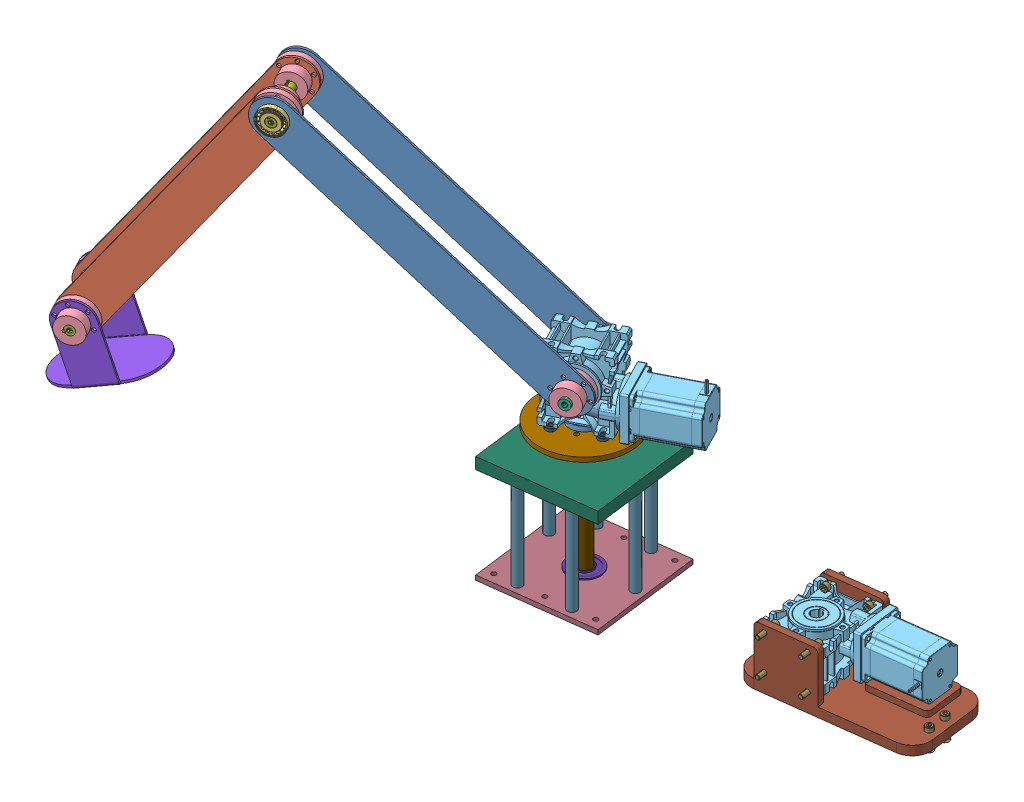
SolidWorks assembly Arm Assembly, configuration Default. Lengths in mm.
Overall size (1001.94 583.28 438.03).
58 component instances, 21 part files, 110 mates.
Components (placement in the parent):
- Link 2-1: Link 2 [Default] at (-10.4598 341.8399 327.9518) x (-0.673407 0.654009 0.344667) z (0.455616 0 0.890177) size (457.2 50.8 3.17)
- Link 3-1: Link 3 [Default] at (-284.4232 603.1069 549.3919) x (-0.514915 -0.815724 0.263547) z (0.455616 0 0.890177) size (406.4 50.8 3.17)
- Flanged Bearing-1: Flanged Bearing [Default] at (-472.9101 298.3431 587.1163) x (0.890177 0 -0.455616) z (0.455616 0 0.890177) size (38.1 38.1 12.7)
- Keyed hub-1: Keyed hub [Default] at (11.7089 322.6251 407.7249) x (0.874279 -0.188145 -0.447479) z (-0.167482 -0.982141 0.085722) size (50.8 25.4 50.8)
- Link 2-2: Link 2 [Default] at (30.1128 341.8399 407.2221) x (-0.673407 0.654009 0.344667) z (0.455616 0 0.890177) size (457.2 50.8 3.17)
- Link 3-2: Link 3 [Default] at (-309.7315 603.1069 499.9449) x (-0.514915 -0.815724 0.263547) z (0.455616 0 0.890177) size (406.4 50.8 3.17)
- Flanged Bearing-2: Flanged Bearing [Default] at (-256.8658 588.4145 557.7576) x (-0.847522 0.30584 0.433784) z (0.455616 0 0.890177) size (38.1 38.1 12.7)
- Flanged Bearing-3: Flanged Bearing [Default] at (-449.1178 298.3431 633.6014) x (-0.822281 -0.383049 0.420865) z (-0.455616 0 -0.890177) size (38.1 38.1 12.7)
- Keyed hub-2: Keyed hub [Default] at (-294.904 588.4145 483.4391) x (0.808999 0.417217 -0.414067) z (0.371397 -0.908807 -0.190091) size (50.8 25.4 50.8)
- Keyed hub-3: Keyed hub [Default] at (-20.1842 322.6251 345.4125) x (-0.874279 0.188145 0.447479) z (-0.167482 -0.982141 0.085722) size (50.8 25.4 50.8)
- Keyed hub-4: Keyed hub [Default] at (-260.9162 588.4145 549.8439) x (-0.808999 -0.417217 0.414067) z (0.371397 -0.908807 -0.190091) size (50.8 25.4 50.8)
- Flanged Bearing-4: Flanged Bearing [Default] at (-298.9544 588.4145 475.5254) x (0.819706 0.38995 -0.419547) z (-0.455616 0 -0.890177) size (38.1 38.1 12.7)
- Nema Stepper Motor-2: Nema Stepper Motor [Default] at (62.3488 303.6559 342.488) x (0.890177 0 -0.455616) z (-0.455616 0 -0.890177) size (171.01 100.01 63.01)
- Keyed Drive Shaft-1: Keyed Drive Shaft [Default] at (-60.5067 325.1756 260.6501) x (0.874279 -0.188145 -0.447479) z (0.455616 0 0.890177) size (19.9 19.9 128.01)
- Keyed Shaft-1: Keyed Shaft [Default] at (-306.0495 588.4145 461.663) x (0.808999 0.417217 -0.414067) z (0.455616 0 0.890177) size (12.7 12.5 104.14)
- Link 4-1: Link 4 [Default] at (-461.4839 217.0007 611.6395) x (0.455616 0 0.890177) z (-0.848146 -0.303649 0.434103) size (90.37 102.6 133.86)
- Keyed hub-5: Keyed hub [Default] at (-476.1168 298.3431 580.8511) x (0.270301 -0.952784 -0.138347) z (0.848146 0.303649 -0.434103) size (50.8 25.4 50.8)
- Keyed hub-6: Keyed hub [Default] at (-445.0674 298.3431 641.515) x (-0.270301 0.952784 0.138347) z (0.848146 0.303649 -0.434103) size (50.8 25.4 50.8)
- Keyed Shaft-2: Keyed Shaft [Default] at (-428.8657 298.3431 673.1697) x (0.270301 -0.952784 -0.138347) z (-0.455616 0 -0.890177) size (12.7 12.5 104.14)
- Joint 2 Motor Plate-1: Joint 2 Motor Plate [Default] at (-4.244 255.2751 376.7854) x (0.954214 0 0.299124) z (-0.299124 0 0.954214) size (127 6.35 127)
- 4 mm M6 spacer-1: 4 mm M6 spacer [94669A162] at (30.7255 263.6251 385.848) x (-0.888418 0 -0.459036) z (0 -1 0) size (13 13 4)
- 4 mm M6 spacer-2: 4 mm M6 spacer [94669A162] at (-17.344 263.6251 410.4513) x (0.999963 0 0.008554) z (0 -1 0) size (13 13 4)
- 4 mm M6 spacer-3: 4 mm M6 spacer [94669A162] at (8.8559 263.6251 343.1196) x (1 0 0) z (0 -1 0) size (13 13 4)
- 4 mm M6 spacer-4: 4 mm M6 spacer [94669A162] at (-39.2136 263.6251 367.7228) x (1 0 0) z (0 -1 0) size (13 13 4)
- Motor Mount Joint 1 Assembly-1: Motor Mount Joint 1 Assembly [Default] at (255.7253 -1.2672 148.6448) x (0.992107 0 -0.125391) z (0.125391 0 0.992107) size (228.6 94.85 140.08)
  - Joint 1 Motor Holder Bracket-1: Joint 1 Motor Holder Bracket [Default] at (55.8829 79.1234 191.166) size (228.6 82.55 114.78)
  - Nema Stepper Motor-1: Nema Stepper Motor [Default] at (81.7887 128.4828 180.6968) x (1 0 0) z (0 1 0) size (171.01 100.01 63.01)
  - Flanged Bearing-1: Flanged Bearing [Default] at (6.9829 88.5722 199.666) x (0.99323 0 0.116162) z (0 -1 0) size (38.1 38.1 12.7)
  - socket head cap screw_am-7: socket head cap screw_am [B18.3.1M - 6 x 1.0 x 25 Hex SHCS -- 25NHX] at (-20.0631 152.4828 153.666) x (0 0 -1) z (0.990069 0.140585 0) size (31 10 10)
  - socket head cap screw_am-8: socket head cap screw_am [B18.3.1M - 6 x 1.0 x 25 Hex SHCS -- 25NHX] at (33.9369 152.4828 228.666) x (0 0 1) z (-1 0 0) size (31 10 10)
  - socket head cap screw_am-9: socket head cap screw_am [B18.3.1M - 6 x 1.0 x 25 Hex SHCS -- 25NHX] at (-20.0631 152.4828 228.666) x (0 0 1) z (0.381849 0.924225 0) size (31 10 10)
  - socket head cap screw_am-10: socket head cap screw_am [B18.3.1M - 6 x 1.0 x 25 Hex SHCS -- 25NHX] at (-20.0631 104.4828 153.666) x (0 0 -1) z (0.756248 0.654286 0) size (31 10 10)
  - socket head cap screw_am-11: socket head cap screw_am [B18.3.1M - 6 x 1.0 x 25 Hex SHCS -- 25NHX] at (33.9369 104.4828 150.5881) x (0 0 -1) z (0.923728 0.383049 0) size (31 10 10)
  - socket head cap screw_am-12: socket head cap screw_am [B18.3.1M - 6 x 1.0 x 25 Hex SHCS -- 25NHX] at (-45.7171 97.8234 212.366) x (0 -1 0) z (-0.546944 0 0.837169) size (31 10 10)
  - socket head cap screw_am-19: socket head cap screw_am [B18.3.1M - 6 x 1.0 x 25 Hex SHCS -- 25NHX] at (-45.7171 97.8234 186.966) x (0 -1 0) z (-0.546944 0 0.837169) size (31 10 10)
  - socket head cap screw_am-14: socket head cap screw_am [B18.3.1M - 6 x 1.0 x 25 Hex SHCS -- 25NHX] at (33.9369 152.4828 153.666) x (0 0 -1) z (0.923728 0.383049 0) size (31 10 10)
  - socket head cap screw_am-15: socket head cap screw_am [B18.3.1M - 6 x 1.0 x 25 Hex SHCS -- 25NHX] at (157.4829 97.8234 186.966) x (0 -1 0) z (-0.546944 0 0.837169) size (31 10 10)
  - socket head cap screw_am-16: socket head cap screw_am [B18.3.1M - 6 x 1.0 x 25 Hex SHCS -- 25NHX] at (-20.0631 104.4828 228.666) x (0 0 1) z (-1 0 0) size (31 10 10)
  - socket head cap screw_am-17: socket head cap screw_am [B18.3.1M - 6 x 1.0 x 25 Hex SHCS -- 25NHX] at (33.9369 104.4828 228.666) x (0 0 1) z (-1 0 0) size (31 10 10)
  - socket head cap screw_am-18: socket head cap screw_am [B18.3.1M - 6 x 1.0 x 25 Hex SHCS -- 25NHX] at (157.4829 97.8234 212.366) x (0 -1 0) z (-0.546944 0 0.837169) size (31 10 10)
- Joint 1 bottom plate-1: Joint 1 bottom plate [89155K113] at (-4.244 81.0311 376.7854) x (-0.125391 0 -0.992107) z (0.992107 0 -0.125391) size (152.4 6.35 152.4)
- Base post-1: Base post [8974K269] at (21.393 160.4061 309.54) x (-0.837169 0 -0.546944) z (0 -1 0) size (12.7 12.7 127)
- Base post-2: Base post [8974K269] at (-29.8811 160.4061 444.0308) x (-0.837169 0 -0.546944) z (0 -1 0) size (12.7 12.7 127)
- Base post-3: Base post [8974K269] at (37.3177 160.4061 435.5376) x (0.463623 0 0.886032) z (0 -1 0) size (12.7 12.7 127)
- Base post-4: Base post [8974K269] at (58.7548 160.4061 368.8231) x (-0.837169 0 -0.546944) z (0 -1 0) size (12.7 12.7 127)
- Base post-5: Base post [8974K269] at (-70.4278 160.4061 359.5483) x (-0.837169 0 -0.546944) z (0 -1 0) size (12.7 12.7 127)
- Base post-6: Base post [8974K269] at (-45.8058 160.4061 318.0332) x (-0.837169 0 -0.546944) z (0 -1 0) size (12.7 12.7 127)
- Base post-7: Base post [8974K269] at (-64.0579 160.4061 409.9473) x (-0.837169 0 -0.546944) z (0 -1 0) size (12.7 12.7 127)
- Joint 1 top plate-1: Joint 1 top plate [89155K143] at (-4.244 219.1436 376.7854) x (-0.125391 0 -0.992107) z (0.992107 0 -0.125391) size (152.4 15.88 152.4)
- Tapered-Roller Bearing-1: Tapered-Roller Bearing [5709K77] at (-4.244 223.5886 376.7854) x (1 0 0) z (0 -1 0) size (45.24 45.24 17.1)
- base Ball Bearing 0.75 in-1: base Ball Bearing 0.75 in [6384K367] at (-4.244 79.4436 376.7854) x (1 0 0) z (0 -1 0) size (44.45 44.45 14.27)
- keyed shaft 0.75 in bore 9 in-1: keyed shaft 0.75 in bore 9 in [Default] at (-4.244 155.2626 376.7854) x (0.954214 0 0.299124) z (0 -1 0) size (19.05 18.75 228.6)
- 0.75 in shaft hub-1: 0.75 in shaft hub [Default] at (-4.244 248.9251 376.7854) x (-0.954214 0 -0.299124) z (0 -1 0) size (63.5 63.5 19.49)
- Clamping Two-Piece Shaft Collar 0.75 in-1: Clamping Two-Piece Shaft Collar 0.75 in [6436K16] at (-4.244 240.9876 376.7854) x (0.996685 0 0.081358) z (0 1 0) size (38.06 38.1 12.77)
- T-slot Slider-1: T-slot Slider [5278N52] at (236.9979 67.7205 365.0672) x (-0.837169 0 -0.546944) z (0 1 0) size (10 9.8 4.82)
- T-slot Slider-2: T-slot Slider [5278N52] at (233.8129 65.4156 339.8677) x (-0.837169 0 -0.546944) z (0 1 0) size (10 9.8 4.82)
- T-slot Slider-3: T-slot Slider [5278N52] at (438.5941 68.7454 339.5877) x (-0.838988 0 -0.544149) z (0 1 0) size (10 9.8 4.82)
- T-slot Slider-4: T-slot Slider [5278N52] at (435.4091 66.889 314.3882) x (-0.837169 0 -0.546944) z (0 1 0) size (10 9.8 4.82)
Mates (geometry in assembly coordinates):
- Concentric3: concentric aligned: cylinder of Keyed hub-1 through (15.3253 322.6251 414.7907) axis (0.455616 0 0.890177) radius 17.4625; cylinder of Link 2-2 through (15.3253 322.6251 414.7907) axis (0.455616 0 0.890177) radius 17.4625
- Coincident2: coincident anti-aligned: plane of Keyed hub-1 through (15.3253 322.6251 414.7907) normal (0.455616 0 0.890177); plane of Link 2-2 through (15.3253 322.6251 414.7907) normal (-0.455616 0 -0.890177)
- Concentric4: concentric aligned: cylinder of Keyed hub-1 through (33.7569 318.6587 405.3569) axis (0.455616 0 0.890177) radius 2.5527; cylinder of Link 2-2 through (35.2035 318.6587 408.1832) axis (0.455616 0 0.890177) radius 2.5527
- Concentric5: concentric anti-aligned: cylinder of Link 2-1 through (-25.2473 322.6251 335.5205) axis (0.455616 0 0.890177) radius 17.4625; cylinder of Keyed hub-3 through (-23.8007 322.6251 338.3468) axis (-0.455616 0 -0.890177) radius 17.4625
- Coincident3: coincident anti-aligned: plane of Link 2-1 through (-23.8007 322.6251 338.3468) normal (0.455616 0 0.890177); plane of Keyed hub-3 through (-23.8007 322.6251 338.3468) normal (-0.455616 0 -0.890177)
- Concentric7: concentric anti-aligned: cylinder of Link 2-1 through (-36.0743 306.6769 344.6287) axis (0.455616 0 0.890177) radius 2.5527; cylinder of Keyed hub-3 through (-36.0743 306.6769 344.6287) axis (-0.455616 0 -0.890177) radius 2.5527
- Concentric8: concentric anti-aligned: cylinder of Keyed hub-1 through (11.7089 322.6251 407.7249) axis (0.455616 0 0.890177) radius 6.35; cylinder of Keyed hub-3 through (-20.1842 322.6251 345.4125) axis (-0.455616 0 -0.890177) radius 6.35
- Coincident5: coincident aligned: plane of Keyed hub-1 through (10.321 322.9238 408.4353) normal (0.874279 -0.188145 -0.447479); plane of Keyed hub-3 through (-21.5721 322.9238 346.1229) normal (0.874279 -0.188145 -0.447479)
- Concentric9: concentric aligned: cylinder of Link 2-2 through (-258.3471 588.4145 554.8634) axis (0.455616 0 0.890177) radius 17.4625; cylinder of Flanged Bearing-2 through (-253.9727 588.4145 563.4102) axis (0.455616 0 0.890177) radius 17.4625
- Concentric10: concentric anti-aligned: cylinder of Link 2-1 through (-298.9197 588.4145 475.5932) axis (0.455616 0 0.890177) radius 17.4625; cylinder of Flanged Bearing-4 through (-301.8476 588.4145 469.8728) axis (-0.455616 0 -0.890177) radius 17.4625
- Concentric11: concentric anti-aligned: cylinder of Link 3-1 through (-265.9793 588.4145 539.9518) axis (0.455616 0 0.890177) radius 17.4625; cylinder of Keyed hub-4 through (-264.5327 588.4145 542.7781) axis (-0.455616 0 -0.890177) radius 17.4625
- Coincident8: coincident anti-aligned: plane of Link 3-1 through (-264.5327 588.4145 542.7781) normal (0.455616 0 0.890177); plane of Keyed hub-4 through (-264.5327 588.4145 542.7781) normal (-0.455616 0 -0.890177)
- Concentric12: concentric anti-aligned: cylinder of Link 3-1 through (-279.8411 600.6092 550.6134) axis (0.455616 0 0.890177) radius 2.5527; cylinder of Keyed hub-4 through (-279.8411 600.6092 550.6134) axis (-0.455616 0 -0.890177) radius 2.5527
- Concentric13: concentric aligned: cylinder of Link 3-2 through (-291.2875 588.4145 490.5048) axis (0.455616 0 0.890177) radius 17.4625; cylinder of Keyed hub-2 through (-291.2875 588.4145 490.5048) axis (0.455616 0 0.890177) radius 17.4625
- Coincident9: coincident anti-aligned: plane of Link 3-2 through (-291.2875 588.4145 490.5048) normal (-0.455616 0 -0.890177); plane of Keyed hub-2 through (-291.2875 588.4145 490.5048) normal (0.455616 0 0.890177)
- Concentric14: concentric aligned: cylinder of Link 3-2 through (-305.1494 600.6092 501.1664) axis (0.455616 0 0.890177) radius 2.5527; cylinder of Keyed hub-2 through (-306.596 600.6092 498.3401) axis (0.455616 0 0.890177) radius 2.5527
- Concentric15: concentric anti-aligned: cylinder of Keyed hub-2 through (-294.904 588.4145 483.4391) axis (0.455616 0 0.890177) radius 6.35; cylinder of Keyed hub-4 through (-260.9162 588.4145 549.8439) axis (-0.455616 0 -0.890177) radius 6.35
- Coincident10: coincident aligned: plane of Keyed hub-2 through (-293.6197 589.0768 482.7817) normal (-0.808999 -0.417217 0.414067); plane of Keyed hub-4 through (-259.632 589.0768 549.1866) normal (-0.808999 -0.417217 0.414067)
- Concentric16: concentric aligned: cylinder of Flanged Bearing-2 through (-253.9727 588.4145 563.4102) axis (0.455616 0 0.890177) radius 6.35; cylinder of Keyed hub-2 through (-294.904 588.4145 483.4391) axis (0.455616 0 0.890177) radius 6.35
- Concentric17: concentric aligned: cylinder of Flanged Bearing-1 through (-470.0169 298.3431 592.769) axis (0.455616 0 0.890177) radius 17.4625; cylinder of Link 3-2 through (-474.3914 298.3431 584.2222) axis (0.455616 0 0.890177) radius 17.4625
- Coincident13: coincident anti-aligned: plane of Flanged Bearing-1 through (-474.3914 315.8056 584.2222) normal (0.455616 0 0.890177); plane of Link 3-2 through (-291.2875 588.4145 490.5048) normal (-0.455616 0 -0.890177)
- Concentric18: concentric anti-aligned: cylinder of Link 3-1 through (-449.0831 298.3431 633.6692) axis (0.455616 0 0.890177) radius 17.4625; cylinder of Flanged Bearing-3 through (-452.011 298.3431 627.9487) axis (-0.455616 0 -0.890177) radius 17.4625
- Coincident14: coincident anti-aligned: plane of Link 3-1 through (-264.5327 588.4145 542.7781) normal (0.455616 0 0.890177); plane of Flanged Bearing-3 through (-453.5909 314.4737 639.5431) normal (-0.455616 0 -0.890177)
- Concentric21: concentric anti-aligned: cylinder of Keyed hub-1 through (11.7089 322.6251 407.7249) axis (0.455616 0 0.890177) radius 6.35; cylinder of Keyed Drive Shaft-1 through (24.9217 322.6251 433.54) axis (-0.455616 0 -0.890177) radius 7
- Parallel1: parallel anti-aligned: plane of Keyed hub-1 through (10.321 322.9238 408.4353) normal (0.874279 -0.188145 -0.447479); plane of Keyed Drive Shaft-1 through (-5.5357 328.3009 377.2331) normal (-0.874279 0.188145 0.447479)
- Coincident18: coincident anti-aligned: plane of Keyed hub-3 through (-20.1842 322.6251 345.4125) normal (0.455616 0 0.890177); plane of Keyed Drive Shaft-1 through (-20.1123 329.4247 345.3758) normal (-0.455616 0 -0.890177)
- Coincident19: coincident anti-aligned: plane of Keyed hub-1 through (11.7089 322.6251 407.7249) normal (-0.455616 0 -0.890177); plane of Keyed Drive Shaft-1 through (11.7808 329.4247 407.6881) normal (0.455616 0 0.890177)
- Concentric22: concentric anti-aligned: cylinder of Keyed hub-2 through (-294.904 588.4145 483.4391) axis (0.455616 0 0.890177) radius 6.35; cylinder of Keyed Shaft-1 through (-253.9727 588.4145 563.4102) axis (-0.455616 0 -0.890177) radius 6.35
- Coincident20: coincident aligned: plane of Keyed hub-2 through (-293.6197 589.0768 482.7817) normal (-0.808999 -0.417217 0.414067); plane of Keyed Shaft-1 through (-254.4524 593.3935 563.6558) normal (-0.808999 -0.417217 0.414067)
- Coincident22: coincident anti-aligned: plane of Link 2-1 through (-23.8007 322.6251 338.3468) normal (0.455616 0 0.890177); plane of Flanged Bearing-4 through (-291.4115 572.3344 475.317) normal (-0.455616 0 -0.890177)
- Distance1: distance = 2.54 mm anti-aligned: plane of Flanged Bearing-4 through (-292.0672 577.8192 479.1337) normal (0.455616 0 0.890177); plane of Keyed hub-2 through (-294.904 588.4145 483.4391) normal (-0.455616 0 -0.890177)
- Coincident24: coincident anti-aligned: plane of Link 2-2 through (15.3253 322.6251 414.7907) normal (-0.455616 0 -0.890177); plane of Flanged Bearing-2 through (-263.1013 571.7887 557.2968) normal (0.455616 0 0.890177)
- Distance2: distance = 2.54 mm anti-aligned: plane of Keyed hub-4 through (-260.9162 588.4145 549.8439) normal (0.455616 0 0.890177); plane of Flanged Bearing-2 through (-262.8916 577.4596 553.7083) normal (-0.455616 0 -0.890177)
- Coincident26: coincident aligned: plane of Flanged Bearing-2 through (-255.7015 582.3687 564.295) normal (0.455616 0 0.890177); plane of Keyed Shaft-1 through (-253.9727 588.4145 563.4102) normal (0.455616 0 0.890177)
- Concentric23: concentric anti-aligned: cylinder of Link 4-1 through (-440.0044 298.3431 651.4071) axis (-0.455616 0 -0.890177) radius 17.4625; cylinder of Keyed hub-6 through (-441.451 298.3431 648.5808) axis (0.455616 0 0.890177) radius 17.4625
- Concentric24: concentric anti-aligned: cylinder of Link 4-1 through (-459.7853 302.8425 657.9648) axis (-0.455616 0 -0.890177) radius 2.5527; cylinder of Keyed hub-6 through (-459.7853 302.8425 657.9648) axis (0.455616 0 0.890177) radius 2.5527
- Coincident27: coincident anti-aligned: plane of Link 4-1 through (-431.2566 177.9232 643.3631) normal (-0.455616 0 -0.890177); plane of Keyed hub-6 through (-441.451 298.3431 648.5808) normal (0.455616 0 0.890177)
- Concentric25: concentric anti-aligned: cylinder of Link 4-1 through (-481.1798 298.3431 570.959) axis (0.455616 0 0.890177) radius 17.4625; cylinder of Keyed hub-5 through (-479.7332 298.3431 573.7853) axis (-0.455616 0 -0.890177) radius 17.4625
- Concentric26: concentric anti-aligned: cylinder of Link 4-1 through (-498.0676 302.8425 583.1693) axis (0.455616 0 0.890177) radius 2.5527; cylinder of Keyed hub-5 through (-498.0676 302.8425 583.1693) axis (-0.455616 0 -0.890177) radius 2.5527
- Concentric27: concentric anti-aligned: cylinder of Keyed hub-5 through (-476.1168 298.3431 580.8511) axis (-0.455616 0 -0.890177) radius 6.35; cylinder of Keyed Shaft-2 through (-480.9426 298.3431 571.4225) axis (0.455616 0 0.890177) radius 6.35
- Coincident31: coincident aligned: plane of Keyed hub-5 through (-476.5459 299.8556 581.0707) normal (0.270301 -0.952784 -0.138347); plane of Keyed Shaft-2 through (-485.4002 298.4134 573.7041) normal (0.270301 -0.952784 -0.138347)
- Coincident32: coincident aligned: plane of Keyed hub-6 through (-433.4948 298.3431 664.1255) normal (0.455616 0 0.890177); plane of Keyed Shaft-2 through (-433.4948 298.3431 664.1255) normal (0.455616 0 0.890177)
- Coincident34: coincident anti-aligned: plane of Link 4-1 through (-469.5389 177.9232 568.5676) normal (0.455616 0 0.890177); plane of Keyed hub-5 through (-479.7332 298.3431 573.7853) normal (-0.455616 0 -0.890177)
- Coincident36: coincident aligned: plane of Keyed hub-6 through (-444.6383 296.8306 641.2954) normal (-0.270301 0.952784 0.138347); plane of Keyed Shaft-2 through (-484.542 295.3883 573.2648) normal (-0.270301 0.952784 0.138347)
- Concentric28: concentric anti-aligned: cone of Flanged Bearing-3 through (-446.5298 298.3431 638.6579) axis (-0.455616 0 -0.890177); cylinder of Keyed Shaft-2 through (-480.9426 298.3431 571.4225) axis (0.455616 0 0.890177) radius 6.35
- Distance3: distance = 2.54 mm anti-aligned: plane of Flanged Bearing-3 through (-450.1481 308.9717 641.2621) normal (0.455616 0 0.890177); plane of Keyed hub-6 through (-445.0674 298.3431 641.515) normal (-0.455616 0 -0.890177)
- Coincident38: coincident anti-aligned: plane of Top base plate-1 through (74.0847 244.0001 261.2257) normal (0 -1 0); plane of arm base spacer small part-1 through (130.8381 244.0001 364.6329) normal (0 1 0)
- Coincident40: coincident anti-aligned: plane of Top base plate-1 through (74.0847 244.0001 261.2257) normal (0 -1 0); plane of arm base spacer large part-1 through (32.1724 244.0001 346.1862) normal (0 1 0)
- Coincident45: coincident anti-aligned: plane of Bearing other part-1 through (32.1724 247.1751 346.1862) normal (0 -1 0); plane of Top base plate-1 through (74.0847 247.1751 261.2257) normal (0 1 0)
- Concentric32: concentric aligned: circle of Bearing other part-1; circle of arm base spacer large part-1
- Coincident57: coincident aligned: plane of Top base plate-1 through (-6.0476 247.1751 446.2586) normal (0.059501 0 0.998228); plane of arm base spacer large part-1 through (84.7912 244.0001 440.844) normal (0.059501 0 0.998228)
- Coincident58: coincident aligned: plane of Top base plate-1 through (-75.7951 247.1751 376.9496) normal (-0.998228 0 0.059501); plane of arm base spacer large part-1 through (-75.8042 244.0001 376.7975) normal (-0.998228 0 0.059501)
- Concentric37: concentric aligned: cylinder of Top base plate-1 through (130.8381 247.1751 364.6329) axis (0 -1 0) radius 15; cylinder of arm base spacer small part-1 through (130.8381 244.0001 364.6329) axis (0 -1 0) radius 15
- Coincident59: coincident aligned: plane of Top base plate-1 through (145.8116 247.1751 363.7404) normal (0.998228 0 -0.059501); plane of arm base spacer small part-1 through (145.8116 244.0001 363.7404) normal (0.998228 0 -0.059501)
- Parallel2: parallel aligned: plane of Nema Stepper Motor-3 through (350.3499 203.0272 320.7095) normal (0 1 0); plane of Top base plate-1 through (74.0847 247.1751 261.2257) normal (0 1 0)
- Parallel3: parallel anti-aligned: plane of Nema Stepper Motor-3 through (312.2058 175.0272 353.0364) normal (-0.998228 0 0.059501); plane of arm base spacer small part-1 through (145.8116 244.0001 363.7404) normal (0.998228 0 -0.059501)
- Coincident61: coincident anti-aligned: plane of Nema Stepper Motor-2 through (44.1227 265.6251 383.271) normal (0 -1 0); plane of 4 mm M6 spacer-1 through (30.7255 265.6251 385.848) normal (0 1 0)
- Concentric43: concentric aligned: cylinder of Keyed hub-1 through (15.3253 322.6251 414.7907) axis (0.455616 0 0.890177) radius 17.4625; cylinder of Nema Stepper Motor-2 through (-46.4848 322.6251 294.0268) axis (0.455616 0 0.890177) radius 7
- Coincident65: coincident anti-aligned: plane of Nema Stepper Motor-2 through (10.1103 322.6251 404.6113) normal (0.455616 0 0.890177); plane of Keyed Drive Shaft-1 through (10.1142 322.6251 404.6093) normal (-0.455616 0 -0.890177)
- Concentric44: concentric aligned: cylinder of Joint 1 bottom plate-1 through (58.7548 83.9521 368.8231) axis (0 1 0) radius 1.905; cylinder of Base post-4 through (58.7548 84.2061 368.8231) axis (0 1 0) radius 6.35
- Concentric45: concentric aligned: cylinder of Joint 1 bottom plate-1 through (37.3177 83.9521 435.5376) axis (0 1 0) radius 1.905; cylinder of Base post-3 through (37.3177 84.2061 435.5376) axis (0 1 0) radius 6.35
- Concentric46: concentric aligned: cylinder of Joint 1 bottom plate-1 through (-29.8811 83.9521 444.0308) axis (0 1 0) radius 1.905; cylinder of Base post-2 through (-29.8811 84.2061 444.0308) axis (0 1 0) radius 6.35
- Concentric47: concentric aligned: cylinder of Joint 1 bottom plate-1 through (21.393 83.9521 309.54) axis (0 1 0) radius 1.905; cylinder of Base post-1 through (21.393 84.2061 309.54) axis (0 1 0) radius 6.35
- Concentric48: concentric aligned: cylinder of Joint 1 bottom plate-1 through (-45.8058 83.9521 318.0332) axis (0 1 0) radius 1.905; cylinder of Base post-6 through (-45.8058 84.2061 318.0332) axis (0 1 0) radius 6.35
- Concentric49: concentric aligned: cylinder of Joint 1 bottom plate-1 through (-64.0579 83.9521 409.9473) axis (0 1 0) radius 1.905; cylinder of Base post-7 through (-64.0579 84.2061 409.9473) axis (0 1 0) radius 6.35
- Concentric50: concentric aligned: cylinder of Joint 1 bottom plate-1 through (-70.4278 83.9521 359.5483) axis (0 1 0) radius 1.905; cylinder of Base post-5 through (-70.4278 84.2061 359.5483) axis (0 1 0) radius 6.35
- Coincident66: coincident anti-aligned: plane of Joint 1 bottom plate-1 through (80.9094 84.2061 442.8292) normal (0 1 0); plane of Base post-4 through (58.7548 84.2061 368.8231) normal (0 -1 0)
- Coincident67: coincident anti-aligned: plane of Joint 1 bottom plate-1 through (80.9094 84.2061 442.8292) normal (0 1 0); plane of Base post-3 through (37.3177 84.2061 435.5376) normal (0 -1 0)
- Coincident68: coincident anti-aligned: plane of Joint 1 bottom plate-1 through (80.9094 84.2061 442.8292) normal (0 1 0); plane of Base post-2 through (-29.8811 84.2061 444.0308) normal (0 -1 0)
- Coincident69: coincident anti-aligned: plane of Joint 1 bottom plate-1 through (80.9094 84.2061 442.8292) normal (0 1 0); plane of Base post-7 through (-64.0579 84.2061 409.9473) normal (0 -1 0)
- Coincident70: coincident anti-aligned: plane of Joint 1 bottom plate-1 through (80.9094 84.2061 442.8292) normal (0 1 0); plane of Base post-1 through (21.393 84.2061 309.54) normal (0 -1 0)
- Coincident71: coincident anti-aligned: plane of Joint 1 bottom plate-1 through (80.9094 84.2061 442.8292) normal (0 1 0); plane of Base post-6 through (-45.8058 84.2061 318.0332) normal (0 -1 0)
- Coincident72: coincident anti-aligned: plane of Joint 1 bottom plate-1 through (80.9094 84.2061 442.8292) normal (0 1 0); plane of Base post-5 through (-70.4278 84.2061 359.5483) normal (0 -1 0)
- Coincident73: coincident aligned: plane of Joint 1 bottom plate-1 through (71.3545 81.0311 367.2306) normal (0.992107 0 -0.125391); plane of Joint 1 top plate-1 through (71.3545 219.1436 367.2306) normal (0.992107 0 -0.125391)
- Coincident74: coincident aligned: plane of Joint 1 bottom plate-1 through (80.9094 77.8561 442.8292) normal (0.125391 0 0.992107); plane of Joint 1 top plate-1 through (80.9094 211.2061 442.8292) normal (0.125391 0 0.992107)
- Coincident75: coincident anti-aligned: plane of Base post-3 through (37.3177 211.2061 435.5376) normal (0 1 0); plane of Joint 1 top plate-1 through (61.7997 211.2061 291.632) normal (0 -1 0)
- Parallel5: parallel aligned: plane of Motor Mount Joint 1 Assembly-1/Joint 1 Motor Holder Bracket-1 through (229.9474 90.5561 403.2135) normal (0.125391 0 0.992107); plane of Joint 1 bottom plate-1 through (80.9094 77.8561 442.8292) normal (0.125391 0 0.992107)
- Coincident79: coincident anti-aligned: plane of Joint 1 top plate-1 through (-4.244 217.5561 376.7854) normal (0 1 0); plane of Tapered-Roller Bearing-1 through (-4.244 217.5561 399.4073) normal (0 -1 0)
- Concentric51: concentric anti-aligned: cylinder of Joint 1 top plate-1 through (-4.244 217.5561 376.7854) axis (0 1 0) radius 22.6219; cylinder of Tapered-Roller Bearing-1 through (-4.244 223.5886 376.7854) axis (0 -1 0) radius 22.6219
- Coincident80: coincident anti-aligned: plane of Nema Stepper Motor-2 through (44.1227 265.6251 383.271) normal (0 -1 0); plane of 4 mm M6 spacer-2 through (-17.344 265.6251 410.4513) normal (0 1 0)
- Coincident81: coincident anti-aligned: plane of Nema Stepper Motor-2 through (44.1227 265.6251 383.271) normal (0 -1 0); plane of 4 mm M6 spacer-4 through (-39.2136 265.6251 367.7228) normal (0 1 0)
- Concentric52: concentric anti-aligned: cylinder of Joint 1 bottom plate-1 through (-4.244 77.8561 376.7854) axis (0 1 0) radius 20.6375; cylinder of base Ball Bearing 0.75 in-1 through (-4.244 73.0936 376.7854) axis (0 -1 0) radius 20.6375
- Coincident82: coincident anti-aligned: plane of Joint 1 bottom plate-1 through (80.9094 84.2061 442.8292) normal (0 1 0); plane of base Ball Bearing 0.75 in-1 through (-4.244 84.2061 395.7927) normal (0 -1 0)
- Concentric53: concentric anti-aligned: cylinder of base Ball Bearing 0.75 in-1 through (-4.244 73.0936 376.7854) axis (0 -1 0) radius 9.525; cylinder of keyed shaft 0.75 in bore-1 through (-4.244 -126.3486 376.7854) axis (0 1 0) radius 9.525
- Concentric54: concentric anti-aligned: cylinder of base Ball Bearing 0.75 in-1 through (-4.244 73.0936 376.7854) axis (0 -1 0) radius 9.525; cylinder of keyed shaft 0.75 in bore 9 in-1 through (-4.244 40.9626 376.7854) axis (0 1 0) radius 9.525
- Coincident83: coincident aligned: plane of Motor Mount Joint 1 Assembly-1/Joint 1 Motor Holder Bracket-1 through (336.1491 77.8561 331.9442) normal (0 -1 0); plane of Joint 1 bottom plate-1 through (61.7997 77.8561 291.632) normal (0 -1 0)
- Concentric55: concentric aligned: cylinder of Joint 2 Motor Plate-1 through (-4.244 255.2751 376.7854) axis (0 1 0) radius 20.6375; circle of 0.75 in shaft hub-1
- Concentric56: concentric anti-aligned: cylinder of Joint 2 Motor Plate-1 through (-16.0098 255.2751 354.2748) axis (0 1 0) radius 3.175; circle of 0.75 in shaft hub-1
- Concentric57: concentric aligned: cylinder of keyed shaft 0.75 in bore 9 in-1 through (-4.244 40.9626 376.7854) axis (0 1 0) radius 9.525; cylinder of 0.75 in shaft hub-1 through (-4.244 247.3376 376.7854) axis (0 1 0) radius 9.525
- Parallel6: parallel aligned: plane of keyed shaft 0.75 in bore 9 in-1 through (-8.6573 40.9626 382.8818) normal (0.954214 0 0.299124); plane of 0.75 in shaft hub-1 through (-10.0777 248.9251 387.4342) normal (0.954214 0 0.299124)
- Coincident90: coincident anti-aligned: plane of Joint 2 Motor Plate-1 through (-4.244 255.2751 376.7854) normal (0 -1 0); plane of 0.75 in shaft hub-1 through (-4.244 255.2751 376.7854) normal (0 1 0)
- Concentric60: concentric anti-aligned: cylinder of keyed shaft 0.75 in bore 9 in-1 through (-4.244 40.9626 376.7854) axis (0 1 0) radius 9.525; cylinder of Clamping Two-Piece Shaft Collar 0.75 in-1 through (-4.244 247.3376 376.7854) axis (0 -1 0) radius 9.525
- Distance7: distance = 1.5875 mm anti-aligned: plane of Tapered-Roller Bearing-1 through (-4.244 233.0501 386.3104) normal (0 1 0); plane of Clamping Two-Piece Shaft Collar 0.75 in-1 through (-4.244 234.6376 376.7854) normal (0 -1 0)
- Distance8: distance = 1.5875 mm anti-aligned: plane of Clamping Two-Piece Shaft Collar 0.75 in-1 through (-4.244 247.3376 376.7854) normal (0 1 0); plane of 0.75 in shaft hub-1 through (-4.244 248.9251 376.7854) normal (0 -1 0)
- Distance9: distance = 1.5875 mm aligned: plane of keyed shaft 0.75 in bore 9 in-1 through (-4.244 269.5626 376.7854) normal (0 1 0); plane of 0.75 in shaft hub-1 through (-4.244 267.9751 376.7854) normal (0 1 0)
- Coincident95: coincident anti-aligned: plane of Nema Stepper Motor-2 through (44.1227 265.6251 383.271) normal (0 -1 0); plane of 4 mm M6 spacer-3 through (8.8559 265.6251 343.1196) normal (0 1 0)
- Coincident96: coincident anti-aligned: plane of Joint 2 Motor Plate-1 through (-4.244 261.6251 376.7854) normal (0 1 0); plane of 4 mm M6 spacer-3 through (8.8559 261.6251 343.1196) normal (0 -1 0)
- Concentric62: concentric anti-aligned: cylinder of Joint 2 Motor Plate-1 through (30.7255 255.2751 385.848) axis (0 1 0) radius 3.25; cylinder of 4 mm M6 spacer-1 through (30.7255 265.6251 385.848) axis (0 -1 0) radius 3.15
- Concentric63: concentric anti-aligned: cylinder of Joint 2 Motor Plate-1 through (-17.344 255.2751 410.4513) axis (0 1 0) radius 3.25; cylinder of 4 mm M6 spacer-2 through (-17.344 265.6251 410.4513) axis (0 -1 0) radius 3.15
- Tangent1: tangent anti-aligned: plane of Nema Stepper Motor-2 through (26.9236 288.3265 385.3337) normal (0.890177 0 -0.455616); cylinder of 4 mm M6 spacer-1 through (30.7255 265.6251 385.848) axis (0 -1 0) radius 3.15
- Tangent2: tangent anti-aligned: plane of Nema Stepper Motor-2 through (-21.1459 288.3265 409.937) normal (0.890177 0 -0.455616); cylinder of 4 mm M6 spacer-2 through (-17.344 265.6251 410.4513) axis (0 -1 0) radius 3.15
- Tangent3: tangent anti-aligned: plane of Nema Stepper Motor-2 through (6.8766 288.3265 346.166) normal (0.890177 0 -0.455616); cylinder of 4 mm M6 spacer-3 through (8.8559 265.6251 343.1196) axis (0 -1 0) radius 3.15
- Concentric67: concentric anti-aligned: cylinder of Joint 2 Motor Plate-1 through (-39.2136 255.2751 367.7228) axis (0 1 0) radius 3.25; cylinder of 4 mm M6 spacer-4 through (-39.2136 265.6251 367.7228) axis (0 -1 0) radius 3.15
- Tangent5: tangent anti-aligned: plane of Nema Stepper Motor-2 through (-41.193 288.3265 370.7692) normal (0.890177 0 -0.455616); cylinder of 4 mm M6 spacer-4 through (-39.2136 265.6251 367.7228) axis (0 -1 0) radius 3.15
- Concentric68: concentric anti-aligned: cylinder of Joint 2 Motor Plate-1 through (8.8559 255.2751 343.1196) axis (0 1 0) radius 3.25; cylinder of 4 mm M6 spacer-3 through (8.8559 265.6251 343.1196) axis (0 -1 0) radius 3.15
- Distance11: distance = 3.81 mm: point of 4 mm M6 spacer-1; plane of Nema Stepper Motor-2 through (8.5157 322.6251 401.4957) normal (0.455616 0 0.890177)
- Concentric69: concentric aligned: cylinder of Motor Mount Joint 1 Assembly-1/socket head cap screw_am-18 through (438.5941 128.3061 339.5877) axis (0 1 0) radius 3; circle of T-slot Slider-3
- Concentric70: concentric aligned: cylinder of Motor Mount Joint 1 Assembly-1/socket head cap screw_am-15 through (435.4091 128.3061 314.3882) axis (0 1 0) radius 3; circle of T-slot Slider-4
- Concentric71: concentric aligned: cylinder of Motor Mount Joint 1 Assembly-1/socket head cap screw_am-12 through (236.9979 128.3061 365.0672) axis (0 1 0) radius 3; circle of T-slot Slider-1
- Concentric72: concentric aligned: cylinder of Motor Mount Joint 1 Assembly-1/socket head cap screw_am-19 through (233.8129 128.3061 339.8677) axis (0 1 0) radius 3; circle of T-slot Slider-2
